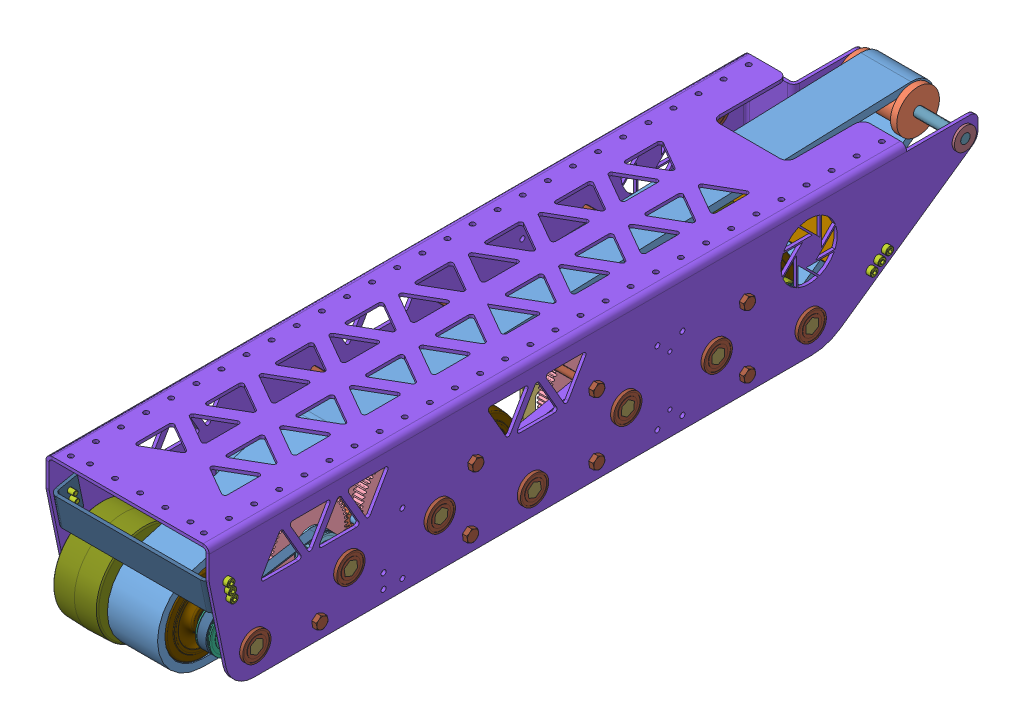
SolidWorks assembly Mirror0001- 01 - 1001 DRIVE TRAIN FRAME NO MATES1, configuration Default. Lengths in mm.
Overall size (218.31 371.92 1576.18).
121 component instances, 30 part files, 18 mates.
Components (placement in the parent):
- 0001- 01 - 0001 Reference Geometry-1: 0001- 01 - 0001 Reference Geometry [Default] at origin size (111.12 355.6 787.4)
- Mirror0001- 01 - 1020 DRIVE ASSEMBLY1-1: Mirror0001- 01 - 1020 DRIVE ASSEMBLY1 [Default] at (102.3557 0 0) size (201.34 355.6 1551.06)
  - 0001- 01 - 0001 Reference Geometry-1: 0001- 01 - 0001 Reference Geometry [Default] at origin size (111.12 355.6 787.4)
  - MirrorMiniCIM1-1: MirrorMiniCIM1 [Default] at (0 75.0243 315.6349) x (-1 0 0) z (0 -0.048874 -0.998805) size (125.82 64.01 64.01)
  - MirrorMiniCIM1-2: MirrorMiniCIM1 [Default] at (0 75.0243 595.7725) x (-1 0 0) z (0 0.532712 0.846296) size (125.82 64.01 64.01)
  - MirrorGear - 11t CIM1-1: MirrorGear - 11t CIM1 [Default] at (13.525 75.0243 315.6349) x (0 -0.998805 0.048874) z (-1 0 0) size (17.96 18.15 19.05)
  - MirrorGear - 11t CIM1-2: MirrorGear - 11t CIM1 [Default] at (13.525 75.0243 595.7725) x (0 0.846296 -0.532712) z (-1 0 0) size (17.96 18.15 19.05)
  - MirrorMiniCIM Washer1-1: MirrorMiniCIM Washer1 [Default] at (23.05 75.0243 315.6349) x (-1 0 0) z (0 -0.066298 -0.9978) size (1.2 14.83 14.83)
  - MirrorMiniCIM Washer1-2: MirrorMiniCIM Washer1 [Default] at (23.05 75.0243 595.7725) x (-1 0 0) z (0 -0.547401 -0.83687) size (1.2 14.83 14.83)
  - MirrorGear - 60t1-1: MirrorGear - 60t1 [Default] at (18.2875 75.0243 269.9149) x (0 0.720477 0.693479) z (1 0 0) size (78.95 78.95 12.65)
  - MirrorGear - 60t1-2: MirrorGear - 60t1 [Default] at (18.2875 75.0243 361.3549) x (0 0.4834 -0.8754) z (1 0 0) size (78.95 78.95 12.65)
  - MirrorGear - 60t1-3: MirrorGear - 60t1 [Default] at (18.2875 75.0243 550.0525) x (0 0.990821 -0.13518) z (1 0 0) size (78.95 78.95 12.65)
  - MirrorGear - 60t1-4: MirrorGear - 60t1 [Default] at (18.2875 75.0243 641.4925) x (0 -0.852945 -0.522001) z (1 0 0) size (78.95 78.95 12.65)
  - MirrorPulley - 18t1-1: MirrorPulley - 18t1 [Default] at (31.8621 75.0243 269.9149) x (0 -0.970691 -0.240332) z (1 0 0) size (32 32 14.5)
  - MirrorPulley - 18t1-2: MirrorPulley - 18t1 [Default] at (31.8621 75.0243 361.3549) x (0 0.8754 0.4834) z (-1 0 0) size (32 32 14.5)
  - MirrorPulley - 18t1-3: MirrorPulley - 18t1 [Default] at (46.3401 75.0243 550.0525) x (0 -0.925666 -0.378341) z (-1 0 0) size (32 32 14.5)
  - MirrorPulley - 18t1-4: MirrorPulley - 18t1 [Default] at (31.8621 75.0243 641.4925) x (0 -0.477672 -0.878538) z (1 0 0) size (32 32 14.5)
  - MirrorPulley - 24t1-1: MirrorPulley - 24t1 [Default] at (31.8621 53.975 174.8073) x (0 0.201275 -0.979535) z (1 0 0) size (42 42 14.5)
  - MirrorPulley - 24t1-2: MirrorPulley - 24t1 [Default] at (31.8621 50.8 455.7037) x (0 0.979669 -0.200622) z (1 0 0) size (42 42 14.5)
  - MirrorPulley - 24t1-3: MirrorPulley - 24t1 [Default] at (31.8621 53.975 736.6) x (0 0.935618 -0.353015) z (1 0 0) size (42 42 14.5)
  - MirrorPulley - 24t1-4: MirrorPulley - 24t1 [Default] at (46.3621 50.8 455.7037) x (0 0.979669 -0.200622) z (1 0 0) size (42 42 14.5)
  - MirrorBelt1-11^Mirror0001- 01 - 1020 DRIVE ASSEMBLY1-1: MirrorBelt1-11^Mirror0001- 01 - 1020 DRIVE ASSEMBLY1 [Default] at (26.3621 57.7677 192.9395) x (0 0 1) z (-1 0 0) size (132.28 58.22 9) (virtual)
  - MirrorBelt2-12^Mirror0001- 01 - 1020 DRIVE ASSEMBLY1-1: MirrorBelt2-12^Mirror0001- 01 - 1020 DRIVE ASSEMBLY1 [Default] at (26.3621 65.6375 351.4578) x (0 0 1) z (-1 0 0) size (131.52 61.39 9) (virtual)
  - MirrorBelt3-13^Mirror0001- 01 - 1020 DRIVE ASSEMBLY1-1: MirrorBelt3-13^Mirror0001- 01 - 1020 DRIVE ASSEMBLY1 [Default] at (40.8621 67.2854 456.4872) x (0 0 1) z (-1 0 0) size (131.52 61.39 9) (virtual)
  - MirrorBelt4-14^Mirror0001- 01 - 1020 DRIVE ASSEMBLY1-1: MirrorBelt4-14^Mirror0001- 01 - 1020 DRIVE ASSEMBLY1 [Default] at (26.3621 71.4781 630.3153) x (0 0 1) z (-1 0 0) size (132.28 58.22 9) (virtual)
- Mirror0001- 01 - 1030 BEARINGS AND AXLES1-1: Mirror0001- 01 - 1030 BEARINGS AND AXLES1 [Default] at origin size (171.45 355.6 1539.56)
  - 0001- 01 - 0001 Reference Geometry-1: 0001- 01 - 0001 Reference Geometry [Default] at origin size (111.12 355.6 787.4)
  - MirrorBearing - 0.5 Hex Flanged1-1: MirrorBearing - 0.5 Hex Flanged1 [Default] at (-3.175 75.0243 641.4925) x (0 0.990292 0.139005) z (0 0.139005 -0.990292) size (31.12 7.94 31.12)
  - MirrorBearing - 0.5 Hex Flanged1-2: MirrorBearing - 0.5 Hex Flanged1 [Default] at (-3.175 53.975 174.8073) x (0 -1 0) z (0 0 1) size (31.12 7.94 31.12)
  - MirrorBearing - 0.5 Hex Flanged1-3: MirrorBearing - 0.5 Hex Flanged1 [Default] at (-3.175 50.8 455.7037) x (0 -0.617689 0.786423) z (0 0.786423 0.617689) size (31.12 7.94 31.12)
  - MirrorBearing - 0.5 Hex Flanged1-4: MirrorBearing - 0.5 Hex Flanged1 [Default] at (-3.175 75.0243 550.0525) x (0 -0.995157 0.098298) z (0 0.098298 0.995157) size (31.12 7.94 31.12)
  - MirrorBearing - 0.5 Hex Flanged1-5: MirrorBearing - 0.5 Hex Flanged1 [Default] at (-3.175 53.975 736.6) x (0 -1 0) z (0 0 1) size (31.12 7.94 31.12)
  - MirrorBearing - 0.5 Hex Flanged1-6: MirrorBearing - 0.5 Hex Flanged1 [Default] at (-3.175 75.0243 269.9149) x (0 -1 0) z (0 0 1) size (31.12 7.94 31.12)
  - MirrorBearing - 0.5 Hex Flanged1-7: MirrorBearing - 0.5 Hex Flanged1 [Default] at (-3.175 75.0243 361.3549) x (0 -0.995055 0.099325) z (0 0.099325 0.995055) size (31.12 7.94 31.12)
  - Mirror0001- 01 - 1031 Hex Axle 6.75x0.51-1: Mirror0001- 01 - 1031 Hex Axle 6.75x0.51 [Default] at (168.275 53.9703 174.8046) x (-1 0 0) z (0 -0.5 0.866025) size (171.45 12.73 14.69)
  - Mirror0001- 01 - 1031 Hex Axle 6.75x0.51-2: Mirror0001- 01 - 1031 Hex Axle 6.75x0.51 [Default] at (-3.175 75.029 269.9176) x (1 0 0) z (0 0.5 0.866025) size (171.45 12.73 14.69)
  - Mirror0001- 01 - 1031 Hex Axle 6.75x0.51-3: Mirror0001- 01 - 1031 Hex Axle 6.75x0.51 [Default] at (-3.175 75.0287 361.3517) x (1 0 0) z (0 -0.41151 0.911405) size (171.45 12.73 14.69)
  - Mirror0001- 01 - 1031 Hex Axle 6.75x0.51-4: Mirror0001- 01 - 1031 Hex Axle 6.75x0.51 [Default] at (-3.175 50.8008 455.6983) x (1 0 0) z (0 -0.372218 -0.928146) size (171.45 12.73 14.69)
  - Mirror0001- 01 - 1031 Hex Axle 6.75x0.51-5: Mirror0001- 01 - 1031 Hex Axle 6.75x0.51 [Default] at (-3.175 75.0225 550.0499) x (1 0 0) z (0 0.582707 0.812682) size (171.45 12.73 14.69)
  - Mirror0001- 01 - 1031 Hex Axle 6.75x0.51-6: Mirror0001- 01 - 1031 Hex Axle 6.75x0.51 [Default] at (-3.175 53.9703 736.5973) x (1 0 0) z (0 -0.5 -0.866025) size (171.45 12.73 14.69)
  - Mirror0001- 01 - 1031 Hex Axle 6.75x0.51-7: Mirror0001- 01 - 1031 Hex Axle 6.75x0.51 [Default] at (-3.175 75.025 641.4871) x (1 0 0) z (0 -0.990292 -0.139005) size (171.45 12.73 14.69)
  - MirrorBearing - 0.5 Hex Flanged1-8: MirrorBearing - 0.5 Hex Flanged1 [Default] at (168.275 53.975 174.8073) x (0 1 0) z (0 0 1) size (31.12 7.94 31.12)
  - MirrorBearing - 0.5 Hex Flanged1-9: MirrorBearing - 0.5 Hex Flanged1 [Default] at (168.275 75.0243 269.9203) x (0 1 0) z (0 0 1) size (31.12 7.94 31.12)
  - MirrorBearing - 0.5 Hex Flanged1-10: MirrorBearing - 0.5 Hex Flanged1 [Default] at (168.275 50.805 455.7017) x (0 -0.989906 -0.141723) z (0 0.141723 -0.989906) size (31.12 7.94 31.12)
  - MirrorBearing - 0.5 Hex Flanged1-11: MirrorBearing - 0.5 Hex Flanged1 [Default] at (168.275 75.0238 361.3495) x (0 -0.995055 0.099325) z (0 -0.099325 -0.995055) size (31.12 7.94 31.12)
  - MirrorBearing - 0.5 Hex Flanged1-12: MirrorBearing - 0.5 Hex Flanged1 [Default] at (168.275 75.0181 550.0531) x (0 0.995157 -0.098298) z (0 0.098298 0.995157) size (31.12 7.94 31.12)
  - MirrorBearing - 0.5 Hex Flanged1-13: MirrorBearing - 0.5 Hex Flanged1 [Default] at (168.275 75.0208 641.4838) x (0 0.990292 0.139005) z (0 -0.139005 0.990292) size (31.12 7.94 31.12)
  - MirrorBearing - 0.5 Hex Flanged1-14: MirrorBearing - 0.5 Hex Flanged1 [Default] at (168.275 53.975 736.6) x (0 1 0) z (0 0 1) size (31.12 7.94 31.12)
  - MirrorBearing - 0.875 Flanged1-1: MirrorBearing - 0.875 Flanged1 [Default] at (46.0375 139.7817 19.05) size (7.11 24.61 24.61)
  - MirrorBearing - 0.875 Flanged1-2: MirrorBearing - 0.875 Flanged1 [Default] at (160.3375 139.7817 19.05) size (7.11 24.61 24.61)
  - Mirror0001- 01 - 1032 Axle 4.75x0.3751-1: Mirror0001- 01 - 1032 Axle 4.75x0.3751 [Default] at (46.7995 139.7817 19.05) x (1 0 0) z (0 -0.031061 0.999517) size (120.65 9.53 9.53)
  - MirrorBearing - 0.5 Hex Flanged1-15: MirrorBearing - 0.5 Hex Flanged1 [Default] at (-3.175 126.365 109.6291) x (0 -1 0) z (0 0 1) size (31.12 7.94 31.12)
- Mirror0001- 01 - 1040 WHEEL ASSEMBLY1-1: Mirror0001- 01 - 1040 WHEEL ASSEMBLY1 [Default] at (4.4625 0 0) size (115.1 371.92 1576.18)
  - 0001- 01 - 0001 Reference Geometry-1: 0001- 01 - 0001 Reference Geometry [Default] at origin size (111.12 355.6 787.4)
  - MirrorColson - 4 x 2 Hex3-1: MirrorColson - 4 x 2 Hex3 [Default] at (28.9766 50.8 455.7037) x (1 0 0) z (0 0.995957 0.089828) size (57.95 99.57 99.57)
    - MirrorColson - 4 x 2 Hex 031-1: MirrorColson - 4 x 2 Hex 031 [Default] at origin size (55.55 82.55 82.55)
    - MirrorColson - 4 x 2 Hex 011-1: MirrorColson - 4 x 2 Hex 011 [Default] at origin size (50.8 99.57 99.57)
    - MirrorColson - 4 x 2 Hex 021-1: MirrorColson - 4 x 2 Hex 021 [Default] x (0 0 -1) z (1 0 0) size (50.79 50.79 57.95)
  - MirrorColson - 4 x 2 Hex31-1: MirrorColson - 4 x 2 Hex31 [Default] at (28.9766 53.975 736.6) x (1 0 0) z (0 0.049345 -0.998782) size (57.95 99.57 99.57)
    - MirrorColson - 4 x 2 Hex 031-1: MirrorColson - 4 x 2 Hex 031 [Default] at origin size (55.55 82.55 82.55)
    - MirrorColson - 4 x 2 Hex 011-1: MirrorColson - 4 x 2 Hex 011 [Default] at origin size (50.8 99.57 99.57)
    - MirrorColson - 4 x 2 Hex 021-1: MirrorColson - 4 x 2 Hex 021 [Default] x (0 0 -1) z (1 0 0) size (50.79 50.79 57.95)
  - MirrorColson - 4 x 2 Hex32-1: MirrorColson - 4 x 2 Hex32 [Default] at (28.9766 53.975 174.8073) x (1 0 0) z (0 -0.745926 -0.666029) size (57.95 99.57 99.57)
    - MirrorColson - 4 x 2 Hex 031-1: MirrorColson - 4 x 2 Hex 031 [Default] at origin size (55.55 82.55 82.55)
    - MirrorColson - 4 x 2 Hex 011-1: MirrorColson - 4 x 2 Hex 011 [Default] at origin size (50.8 99.57 99.57)
    - MirrorColson - 4 x 2 Hex 021-1: MirrorColson - 4 x 2 Hex 021 [Default] x (0 0 -1) z (1 0 0) size (50.79 50.79 57.95)
  - MirrorColson - 3 x 0.875 Hex1-1: MirrorColson - 3 x 0.875 Hex1 [Default] at (71.7469 53.975 174.8073) x (0 0.203834 -0.979005) z (1 0 0) size (76.2 76.2 27.59)
  - MirrorColson - 3 x 0.875 Hex1-2: MirrorColson - 3 x 0.875 Hex1 [Default] at (99.3345 53.975 174.8073) x (0 0.203834 -0.979005) z (1 0 0) size (76.2 76.2 27.59)
  - MirrorColson - 3 x 0.875 Hex1-3: MirrorColson - 3 x 0.875 Hex1 [Default] at (71.7469 50.8 455.7037) x (0 -0.995957 -0.089828) z (1 0 0) size (76.2 76.2 27.59)
  - MirrorColson - 3 x 0.875 Hex1-4: MirrorColson - 3 x 0.875 Hex1 [Default] at (99.3345 50.8 455.7037) x (0 -0.995957 -0.089828) z (1 0 0) size (76.2 76.2 27.59)
  - MirrorColson - 3 x 0.875 Hex1-5: MirrorColson - 3 x 0.875 Hex1 [Default] at (99.3345 53.975 736.6) x (0 -0.049345 0.998782) z (1 0 0) size (76.2 76.2 27.59)
  - MirrorColson - 3 x 0.875 Hex1-6: MirrorColson - 3 x 0.875 Hex1 [Default] at (71.7469 53.975 736.6) x (0 -0.049345 0.998782) z (1 0 0) size (76.2 76.2 27.59)
  - Mirror0001- 01 - 1041 Tread1-1: Mirror0001- 01 - 1041 Tread1 [Default] at (57.9532 0 0) size (50.8 157.69 786.26)
  - Mirror0001- 01 - 1042 Top Pulley1-1: Mirror0001- 01 - 1042 Top Pulley1 [Default] at (51.6032 139.7817 19.05) x (1 0 0) z (0 -0.762622 0.646844) size (63.5 43.18 43.18)
- Mirror0001- 01 - 1050 MOUNTING ASSEMBLY1-1: Mirror0001- 01 - 1050 MOUNTING ASSEMBLY1 [Default] at (102.3557 0 0) size (171.45 355.6 1472.66)
  - 0001- 01 - 0001 Reference Geometry-1: 0001- 01 - 0001 Reference Geometry [Default] at origin size (111.12 355.6 787.4)
  - Mirror0001- 01 - 1051 CIM Mounting Plate1-1: Mirror0001- 01 - 1051 CIM Mounting Plate1 [Default] at origin size (3.17 88.9 177.8)
  - Mirror0001- 01 - 1052 CIM Mounting Plate Back1-1: Mirror0001- 01 - 1052 CIM Mounting Plate Back1 [Default] at origin size (3.18 85.92 177.8)
  - Mirror0001- 01 - 1053 CIM Mounting Plate Outer1-1: Mirror0001- 01 - 1053 CIM Mounting Plate Outer1 [Default] at (-55.5625 0 0) size (3.18 88.9 177.8)
  - Mirror0001- 01 - 1054 CIM Mounting Plate Outer Back1-1: Mirror0001- 01 - 1054 CIM Mounting Plate Outer Back1 [Default] at (-55.5625 6.3555 0.5906) size (3.18 80.08 177.8)
  - socket head cap screw_ai-1: socket head cap screw_ai [HX-SHCS 0.19-32x2.5x1.125-N] at (9.5885 36.9243 586.2475) x (-1 0 0) z (0 -0.924225 0.381849) size (68.33 7.94 7.94)
  - socket head cap screw_ai-2: socket head cap screw_ai [HX-SHCS 0.19-32x2.5x1.125-N] at (9.5885 36.9243 605.2975) x (-1 0 0) z (0 -0.924225 0.381849) size (68.33 7.94 7.94)
  - socket head cap screw_ai-3: socket head cap screw_ai [HX-SHCS 0.19-32x2.5x1.125-N] at (8.001 38.1943 302.9349) x (-1 0 0) z (0 -0.924225 0.381849) size (68.33 7.94 7.94)
  - socket head cap screw_ai-4: socket head cap screw_ai [HX-SHCS 0.19-32x2.5x1.125-N] at (8.001 38.1943 328.3349) x (-1 0 0) z (0 -0.924225 0.381849) size (68.33 7.94 7.94)
  - socket head cap screw_ai-5: socket head cap screw_ai [HX-SHCS 0.19-32x2.5x1.125-N] at (8.001 111.8543 328.3349) x (-1 0 0) z (0 -0.924225 0.381849) size (68.33 7.94 7.94)
  - socket head cap screw_ai-6: socket head cap screw_ai [HX-SHCS 0.19-32x2.5x1.125-N] at (8.001 111.8543 302.9349) x (-1 0 0) z (0 -0.924225 0.381849) size (68.33 7.94 7.94)
  - socket head cap screw_ai-7: socket head cap screw_ai [HX-SHCS 0.19-32x0.5x0.5-N] at (9.5885 98.5707 586.2475) x (-1 0 0) z (0 -0.924225 0.381849) size (17.53 7.94 7.94)
  - socket head cap screw_ai-8: socket head cap screw_ai [HX-SHCS 0.19-32x0.5x0.5-N] at (9.5885 51.4779 605.2975) x (-1 0 0) z (0 -0.924225 0.381849) size (17.53 7.94 7.94)
  - socket head cap screw_ai-9: socket head cap screw_ai [HX-SHCS 0.19-32x0.5x0.5-N] at (8.001 49.6243 315.6349) x (-1 0 0) z (0 -0.924225 0.381849) size (17.53 7.94 7.94)
  - socket head cap screw_ai-10: socket head cap screw_ai [HX-SHCS 0.19-32x0.5x0.5-N] at (8.001 100.4243 315.6349) x (-1 0 0) z (0 -0.924225 0.381849) size (17.53 7.94 7.94)
- Mirror0001- 01 - 1060 FRAME ASSEMBLY1-1: Mirror0001- 01 - 1060 FRAME ASSEMBLY1 [Default] at origin size (174.75 355.6 1569.05)
  - 0001- 01 - 0001 Reference Geometry-1: 0001- 01 - 0001 Reference Geometry [Default] at origin size (111.12 355.6 787.4)
  - Mirror0001- 01 - 1010 Drive Frame1-1: Mirror0001- 01 - 1010 Drive Frame1 [Default] at origin size (165.1 136.61 777.68)
  - Mirror0001- 01 - 1011 Frame Support Front1-1: Mirror0001- 01 - 1011 Frame Support Front1 [Default] at (3.175 0 0) size (158.75 37.46 42.14)
  - Mirror0001- 01 - 1012 Frame Support Back1-1: Mirror0001- 01 - 1012 Frame Support Back1 [Default] at (3.175 0 0) size (158.75 36.23 31.29)
  - socket head cap screw_ai-1: socket head cap screw_ai [HX-SHCS 0.19-32x0.5x0.5-N] at (169.926 123.8969 763.9866) x (-1 0 0) z (0 -0.924225 0.381849) size (17.53 7.94 7.94)
  - socket head cap screw_ai-2: socket head cap screw_ai [HX-SHCS 0.19-32x0.5x0.5-N] at (169.926 116.123 762.3835) x (-1 0 0) z (0 -0.924225 0.381849) size (17.53 7.94 7.94)
  - socket head cap screw_ai-3: socket head cap screw_ai [HX-SHCS 0.19-32x0.5x0.5-N] at (169.926 108.3491 760.7803) x (-1 0 0) z (0 -0.924225 0.381849) size (17.53 7.94 7.94)
  - socket head cap screw_ai-4: socket head cap screw_ai [HX-SHCS 0.19-32x0.5x0.5-N] at (-4.826 123.8969 763.9866) size (17.53 7.94 7.94)
  - socket head cap screw_ai-5: socket head cap screw_ai [HX-SHCS 0.19-32x0.5x0.5-N] at (-4.826 116.123 762.3835) size (17.53 7.94 7.94)
  - socket head cap screw_ai-6: socket head cap screw_ai [HX-SHCS 0.19-32x0.5x0.5-N] at (-4.826 108.3491 760.7803) size (17.53 7.94 7.94)
  - socket head cap screw_ai-7: socket head cap screw_ai [HX-SHCS 0.19-32x0.5x0.5-N] at (-4.826 81.7927 97.7153) x (1 0 0) z (0 0.557697 0.830044) size (17.53 7.94 7.94)
  - socket head cap screw_ai-8: socket head cap screw_ai [HX-SHCS 0.19-32x0.5x0.5-N] at (-4.826 76.3294 105.5177) size (17.53 7.94 7.94)
  - socket head cap screw_ai-9: socket head cap screw_ai [HX-SHCS 0.19-32x0.5x0.5-N] at (-4.826 70.8661 113.3202) size (17.53 7.94 7.94)
  - socket head cap screw_ai-10: socket head cap screw_ai [HX-SHCS 0.19-32x0.5x0.5-N] at (169.926 81.7927 97.7153) x (-1 0 0) z (0 -0.924225 0.381849) size (17.53 7.94 7.94)
  - socket head cap screw_ai-11: socket head cap screw_ai [HX-SHCS 0.19-32x0.5x0.5-N] at (169.926 76.3294 105.5177) x (-1 0 0) z (0 -0.924225 0.381849) size (17.53 7.94 7.94)
  - socket head cap screw_ai-12: socket head cap screw_ai [HX-SHCS 0.19-32x0.5x0.5-N] at (169.926 70.8661 113.3202) x (-1 0 0) z (0 -0.924225 0.381849) size (17.53 7.94 7.94)
  - hex bolt_ai-1: hex bolt_ai [HBOLT 0.2500-20x2.5x0.75-N] at (169.8752 106.7743 239.4349) x (-1 0 0) z (0 -0.924225 0.381849) size (68.28 12.85 11.13)
  - hex bolt_ai-2: hex bolt_ai [HBOLT 0.2500-20x2.5x0.75-N] at (169.8752 106.7743 391.8349) x (-1 0 0) z (0 -0.924225 0.381849) size (68.28 12.85 11.13)
  - hex bolt_ai-3: hex bolt_ai [HBOLT 0.2500-20x2.5x0.75-N] at (169.8752 43.2743 391.8349) x (-1 0 0) z (0 -0.924225 0.381849) size (68.28 12.85 11.13)
  - hex bolt_ai-4: hex bolt_ai [HBOLT 0.2500-20x2.5x0.75-N] at (169.8752 43.2743 239.4349) x (-1 0 0) z (0 -0.924225 0.381849) size (68.28 12.85 11.13)
  - hex bolt_ai-5: hex bolt_ai [HBOLT 0.2500-20x2.5x0.75-N] at (169.8752 102.9745 514.2182) x (-1 0 0) z (0 -0.924225 0.381849) size (68.28 12.85 11.13)
  - hex bolt_ai-6: hex bolt_ai [HBOLT 0.2500-20x2.5x0.75-N] at (169.8752 43.2743 519.5725) x (-1 0 0) z (0 -0.924225 0.381849) size (68.28 12.85 11.13)
  - hex bolt_ai-7: hex bolt_ai [HBOLT 0.2500-20x2.5x0.75-N] at (169.8752 43.2743 671.9725) x (-1 0 0) z (0 -0.924225 0.381849) size (68.28 12.85 11.13)
  - hex bolt_ai-8: hex bolt_ai [HBOLT 0.2500-20x2x2-N] at (-4.7752 106.7743 239.4349) size (55.58 12.85 11.13)
  - hex bolt_ai-9: hex bolt_ai [HBOLT 0.2500-20x2x2-N] at (-4.7752 43.2743 239.4349) size (55.58 12.85 11.13)
  - hex bolt_ai-10: hex bolt_ai [HBOLT 0.2500-20x2x2-N] at (-4.7752 43.2743 391.8349) size (55.58 12.85 11.13)
  - hex bolt_ai-11: hex bolt_ai [HBOLT 0.2500-20x2x2-N] at (-4.7752 106.7743 391.8349) size (55.58 12.85 11.13)
  - hex bolt_ai-12: hex bolt_ai [HBOLT 0.2500-20x2x2-N] at (-4.7752 102.9745 514.2182) size (55.58 12.85 11.13)
  - hex bolt_ai-13: hex bolt_ai [HBOLT 0.2500-20x2x2-N] at (-4.7752 43.2743 519.5725) size (55.58 12.85 11.13)
  - hex bolt_ai-14: hex bolt_ai [HBOLT 0.2500-20x2x2-N] at (-4.7752 43.2743 671.9725) size (55.58 12.85 11.13)
Mates (geometry in assembly coordinates):
- Coincident1: coincident aligned: plane of 0001- 01 - 0001 Reference Geometry-1 through (0 0 0) normal (0 0 1); plane of assembly through (0 0 0) normal (0 0 1)
- Coincident2: coincident aligned: plane of 0001- 01 - 0001 Reference Geometry-1 through (0 0 0) normal (0 1 0); plane of assembly through (0 0 0) normal (0 1 0)
- Coincident3: coincident aligned: plane of 0001- 01 - 0001 Reference Geometry-1 through (0 0 0) normal (1 0 0); plane of assembly through (0 0 0) normal (1 0 0)
- Coincident4: coincident aligned: plane of Mirror0001- 01 - 1020 DRIVE ASSEMBLY1-1/0001- 01 - 0001 Reference Geometry-1 through (102.3557 0 0) normal (0 0 1); plane of assembly through (0 0 0) normal (0 0 1)
- Coincident5: coincident aligned: plane of Mirror0001- 01 - 1020 DRIVE ASSEMBLY1-1/0001- 01 - 0001 Reference Geometry-1 through (102.3557 0 0) normal (0 1 0); plane of assembly through (0 0 0) normal (0 1 0)
- Coincident6: coincident aligned: plane of Mirror0001- 01 - 1030 BEARINGS AND AXLES1-1/0001- 01 - 0001 Reference Geometry-1 through (0 0 0) normal (0 0 1); plane of assembly through (0 0 0) normal (0 0 1)
- Coincident7: coincident aligned: plane of Mirror0001- 01 - 1030 BEARINGS AND AXLES1-1/0001- 01 - 0001 Reference Geometry-1 through (0 0 0) normal (0 1 0); plane of assembly through (0 0 0) normal (0 1 0)
- Coincident8: coincident aligned: plane of Mirror0001- 01 - 1030 BEARINGS AND AXLES1-1/0001- 01 - 0001 Reference Geometry-1 through (0 0 0) normal (1 0 0); plane of assembly through (0 0 0) normal (1 0 0)
- Coincident9: coincident aligned: plane of Mirror0001- 01 - 1040 WHEEL ASSEMBLY1-1/0001- 01 - 0001 Reference Geometry-1 through (4.4625 0 0) normal (0 0 1); plane of assembly through (0 0 0) normal (0 0 1)
- Coincident10: coincident aligned: plane of Mirror0001- 01 - 1040 WHEEL ASSEMBLY1-1/0001- 01 - 0001 Reference Geometry-1 through (4.4625 0 0) normal (0 1 0); plane of assembly through (0 0 0) normal (0 1 0)
- Coincident11: coincident anti-aligned: plane of Mirror0001- 01 - 1030 BEARINGS AND AXLES1-1/MirrorBearing - 0.5 Hex Flanged1-2 through (4.7625 41.275 174.8073) normal (1 0 0); plane of Mirror0001- 01 - 1040 WHEEL ASSEMBLY1-1/MirrorColson - 4 x 2 Hex32-1/MirrorColson - 4 x 2 Hex 021-1 through (4.7625 53.975 174.8073) normal (-1 0 0)
- Coincident12: coincident aligned: plane of ? through (102.3557 0 0) normal (0 0 1); plane of assembly through (0 0 0) normal (0 0 1)
- Coincident13: coincident aligned: plane of ? through (102.3557 0 0) normal (0 1 0); plane of assembly through (0 0 0) normal (0 1 0)
- Coincident14: coincident anti-aligned: plane of Mirror0001- 01 - 1020 DRIVE ASSEMBLY1-1/MirrorMiniCIM1-1 through (102.3557 84.5379 315.1693) normal (1 0 0); plane of ? through (102.3557 106.7743 239.4349) normal (-1 0 0)
- Coincident15: coincident aligned: plane of ? through (0 0 0) normal (0 0 1); plane of assembly through (0 0 0) normal (0 0 1)
- Coincident16: coincident aligned: plane of ? through (0 0 0) normal (1 0 0); plane of assembly through (0 0 0) normal (1 0 0)
- Coincident17: coincident aligned: plane of ? through (0 0 0) normal (0 1 0); plane of assembly through (0 0 0) normal (0 1 0)
- Coincident18: coincident anti-aligned: plane of ? through (102.3557 106.7743 239.4349) normal (-1 0 0); circle of Mirror0001- 01 - 1060 FRAME ASSEMBLY1-1/hex bolt_ai-1
